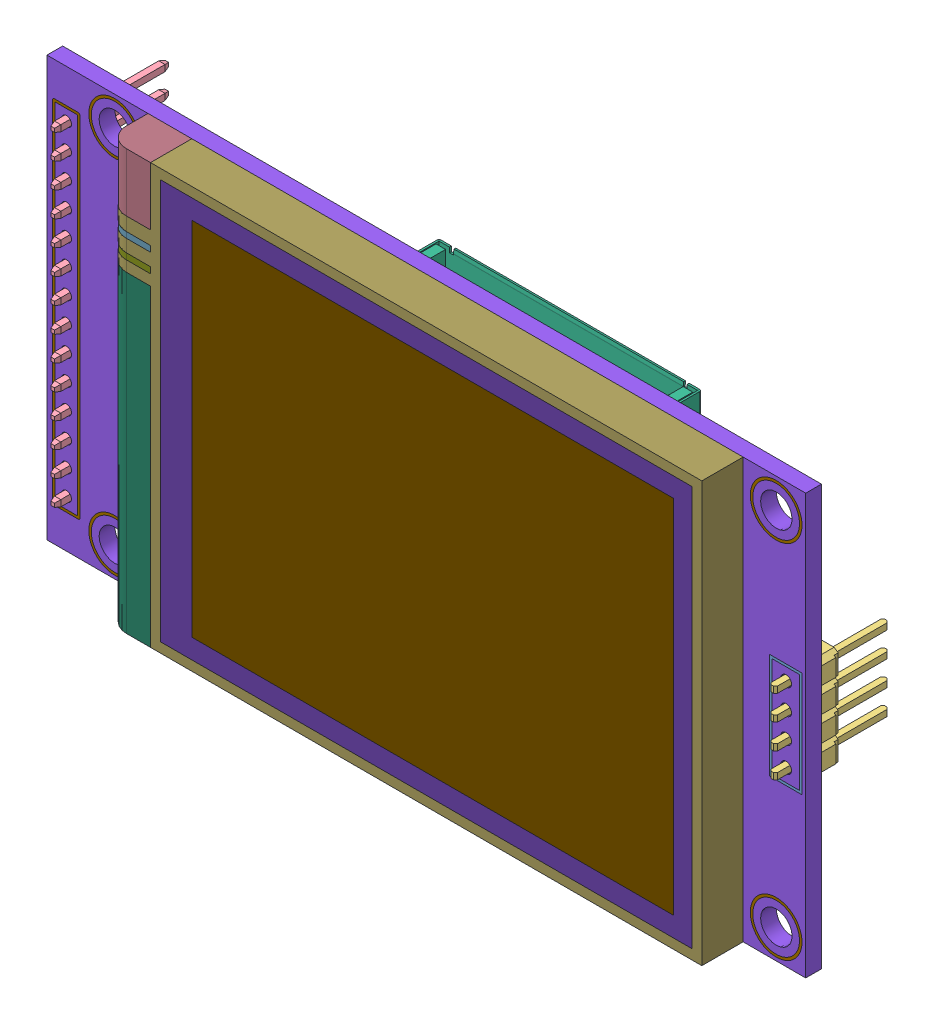
SolidWorks assembly TFT LCD 2.4 inch ILI9341 touch, configuration Default. Lengths in mm.
Overall size (77.15 42.7 14.4).
41 component instances, 19 part files, 0 mates.
Components (placement in the parent):
- TFT LCD 2.4 inch ILI9341 touch.step-1: TFT LCD 2.4 inch ILI9341 touch.step [Default] at origin size (77.15 42.7 14.4)
  - R1~R0603~R0603~HwOR.step-1: R1~R0603~R0603~HwOR.step [Default] at (51.3313 17.8702 0) x (0 -1 0) z (0 0 -1) size (1.62 0.81 0.45)
    - R0603~R0603~HwOR.step-1: R0603~R0603~HwOR.step [Default] at origin size (1.62 0.81 0.45)
  - C1~C0603~C0603_L1.6-W0.8-H0.8~HwOR.step-1: C1~C0603~C0603_L1.6-W0.8-H0.8~HwOR.step [Default] at (30.0394 8.9761 0) x (1 0 0) z (0 0 -1) size (1.6 0.8 0.8)
    - C0603~C0603_L1.6-W0.8-H0.8~HwOR.step-1: C0603~C0603_L1.6-W0.8-H0.8~HwOR.step [Default] at origin size (1.6 0.8 0.8)
  - H2~HDR-TH_4P-P2.54-V-M~HDR-TH_4P-P2.54-M-LI-1X4P~HwOR.step-1: H2~HDR-TH_4P-P2.54-V-M~HDR-TH_4P-P2.54-M-LI-1X4P~HwOR.step [Default] at (75.1801 25.1701 0) x (0 -1 0) z (0 0 -1) size (10.17 2.66 11.54)
    - HDR-TH_4P-P2.54-V-M~HDR-TH_4P-P2.54-M-LI-1X4P~HwOR.step-1: HDR-TH_4P-P2.54-V-M~HDR-TH_4P-P2.54-M-LI-1X4P~HwOR.step [Default] at origin size (10.17 2.66 11.54)
  - H3~CONN-TH_PZ254V-11-14P~CONN-TH_PZ254V-11-14P~HwOR.step-1: H3~CONN-TH_PZ254V-11-14P~CONN-TH_PZ254V-11-14P~HwOR.step [Default] at (2 4.85 0) x (0 1 0) z (0 0 -1) size (35.57 2.5 11.6)
    - CONN-TH_PZ254V-11-14P~CONN-TH_PZ254V-11-14P~HwOR.step-1: CONN-TH_PZ254V-11-14P~CONN-TH_PZ254V-11-14P~HwOR.step [Default] at origin size (35.57 2.5 11.6)
  - Q1~SOT-23-3_L2.9-W1.3-P1.90-LS2.4-BR~SOT-23-3P_L2.9-W1.3-H1.0-LS2.4-P0.95~HwOR.step-1: Q1~SOT-23-3_L2.9-W1.3-P1.90-LS2.4-BR~SOT-23-3P_L2.9-W1.3-H1.0-LS2.4-P0.95~HwOR.step [Default] at (19.5843 21.1653 0) x (-1 0 0) z (0 0 -1) size (2.5 2.89 1.06)
    - SOT-23-3_L2.9-W1.3-P1.90-LS2.4-BR~SOT-23-3P_L2.9-W1.3-H1.0-LS2.4-P0.95~HwOR.step-1: SOT-23-3_L2.9-W1.3-P1.90-LS2.4-BR~SOT-23-3P_L2.9-W1.3-H1.0-LS2.4-P0.95~HwOR.step [Default] at origin size (2.5 2.89 1.06)
  - U1~SD-CARD-SMD_SD-CARD-11P~SD-CARD-SMD_SD-CARD-11P~HwOR.step-1: U1~SD-CARD-SMD_SD-CARD-11P~SD-CARD-SMD_SD-CARD-11P~HwOR.step [Default] at (48.7311 32.7935 0) x (1 0 0) z (0 0 -1) size (27.7 17.71 3.85)
    - SD-CARD-SMD_SD-CARD-11P~SD-CARD-SMD_SD-CARD-11P~HwOR.step-1: SD-CARD-SMD_SD-CARD-11P~SD-CARD-SMD_SD-CARD-11P~HwOR.step [Default] at origin size (27.7 17.71 3.85)
  - U2~TSSOP-16_L5.0-W4.4-P0.65-LS6.4-BL~TSSOP-16_L5.0-W4.4-H1.0-LS6.4-P0.65~HwOR.step-1: U2~TSSOP-16_L5.0-W4.4-P0.65-LS6.4-BL~TSSOP-16_L5.0-W4.4-H1.0-LS6.4-P0.65~HwOR.step [Default] at (22.8993 6.6301 0) x (0 -1 0) z (0 0 -1) size (5 6.41 1.05)
    - TSSOP-16_L5.0-W4.4-P0.65-LS6.4-BL~TSSOP-16_L5.0-W4.4-H1.0-LS6.4-P0.65~HwOR.step-1: TSSOP-16_L5.0-W4.4-P0.65-LS6.4-BL~TSSOP-16_L5.0-W4.4-H1.0-LS6.4-P0.65~HwOR.step [Default] at origin size (5 6.41 1.05)
  - R1~R0603~R0603~HwOR.step-2: R1~R0603~R0603~HwOR.step [Default] at (48.6536 17.8702 0) x (0 -1 0) z (0 0 -1) size (1.62 0.81 0.45)
    - R0603~R0603~HwOR.step-1: R0603~R0603~HwOR.step [Default] at origin size (1.62 0.81 0.45)
  - R1~R0603~R0603~HwOR.step-3: R1~R0603~R0603~HwOR.step [Default] at (45.9973 17.8702 0) x (0 -1 0) z (0 0 -1) size (1.62 0.81 0.45)
    - R0603~R0603~HwOR.step-1: R0603~R0603~HwOR.step [Default] at origin size (1.62 0.81 0.45)
  - R1~R0603~R0603~HwOR.step-4: R1~R0603~R0603~HwOR.step [Default] at (16.535 21.1653 0) x (0 -1 0) z (0 0 -1) size (1.62 0.81 0.45)
    - R0603~R0603~HwOR.step-1: R0603~R0603~HwOR.step [Default] at origin size (1.62 0.81 0.45)
  - R1~R0603~R0603~HwOR.step-5: R1~R0603~R0603~HwOR.step [Default] at (16.6772 4.0801 0) x (0 -1 0) z (0 0 -1) size (1.62 0.81 0.45)
    - R0603~R0603~HwOR.step-1: R0603~R0603~HwOR.step [Default] at origin size (1.62 0.81 0.45)
  - R1~R0603~R0603~HwOR.step-6: R1~R0603~R0603~HwOR.step [Default] at (22.9395 21.1858 0) x (0 -1 0) z (0 0 -1) size (1.62 0.81 0.45)
    - R0603~R0603~HwOR.step-1: R0603~R0603~HwOR.step [Default] at origin size (1.62 0.81 0.45)
  - C1~C0603~C0603_L1.6-W0.8-H0.8~HwOR.step-2: C1~C0603~C0603_L1.6-W0.8-H0.8~HwOR.step [Default] at (22.7962 15.1258 0) x (0 -1 0) z (0 0 -1) size (1.6 0.8 0.8)
    - C0603~C0603_L1.6-W0.8-H0.8~HwOR.step-1: C0603~C0603_L1.6-W0.8-H0.8~HwOR.step [Default] at origin size (1.6 0.8 0.8)
  - Q1~SOT-23-3_L2.9-W1.3-P1.90-LS2.4-BR~SOT-23-3P_L2.9-W1.3-H1.0-LS2.4-P0.95~HwOR.step-2: Q1~SOT-23-3_L2.9-W1.3-P1.90-LS2.4-BR~SOT-23-3P_L2.9-W1.3-H1.0-LS2.4-P0.95~HwOR.step [Default] at (19.3803 15.2492 0) x (0 1 0) z (0 0 -1) size (2.5 2.89 1.06)
    - SOT-23-3_L2.9-W1.3-P1.90-LS2.4-BR~SOT-23-3P_L2.9-W1.3-H1.0-LS2.4-P0.95~HwOR.step-1: SOT-23-3_L2.9-W1.3-P1.90-LS2.4-BR~SOT-23-3P_L2.9-W1.3-H1.0-LS2.4-P0.95~HwOR.step [Default] at origin size (2.5 2.89 1.06)
  - Board~HwOR.step-1: Board~HwOR.step [Default] at origin size (77.15 42.69 1.6)
  - TopSilkscreen~HwOR.step-1: TopSilkscreen~HwOR.step [Default] at (0 0 1.6201) size (76.19 42.7 0.01)
  - BottomSilkscreen~HwOR.step-1: BottomSilkscreen~HwOR.step [Default] at (0 0 -0.02) size (75.96 41.18 0.02)
  - text.step-1: text.step [Default] at origin size (2.87 0.1 1)
  - EasyEDA PCB Model~HwOR.step-1: EasyEDA PCB Model~HwOR.step [Default] at origin size (60.51 42.69 4.2)
  - EasyEDA PCB Model~HwOR-0.step-1: EasyEDA PCB Model~HwOR-0.step [Default] at origin size (4.46 5.93 4.2)
  - EasyEDA PCB Model~HwOR-1.step-1: EasyEDA PCB Model~HwOR-1.step [Default] at origin size (4.45 0.59 4.2)
  - EasyEDA PCB Model~HwOR-2.step-1: EasyEDA PCB Model~HwOR-2.step [Default] at origin size (4.45 31.81 4.2)
  - EasyEDA PCB Model~HwOR-3.step-1: EasyEDA PCB Model~HwOR-3.step [Default] at origin size (4.45 0.62 4.2)
  - EasyEDA PCB Model~HwOR-4.step-1: EasyEDA PCB Model~HwOR-4.step [Default] at origin size (54.06 40.69 4.2)
  - EasyEDA PCB Model~HwOR-5.step-1: EasyEDA PCB Model~HwOR-5.step [Default] at origin size (48.96 36.72 4.2)
  - EasyEDA PCB Model~HwOR-6.step-1: EasyEDA PCB Model~HwOR-6.step [Default] at origin size (3.3 10.72 0.1)
